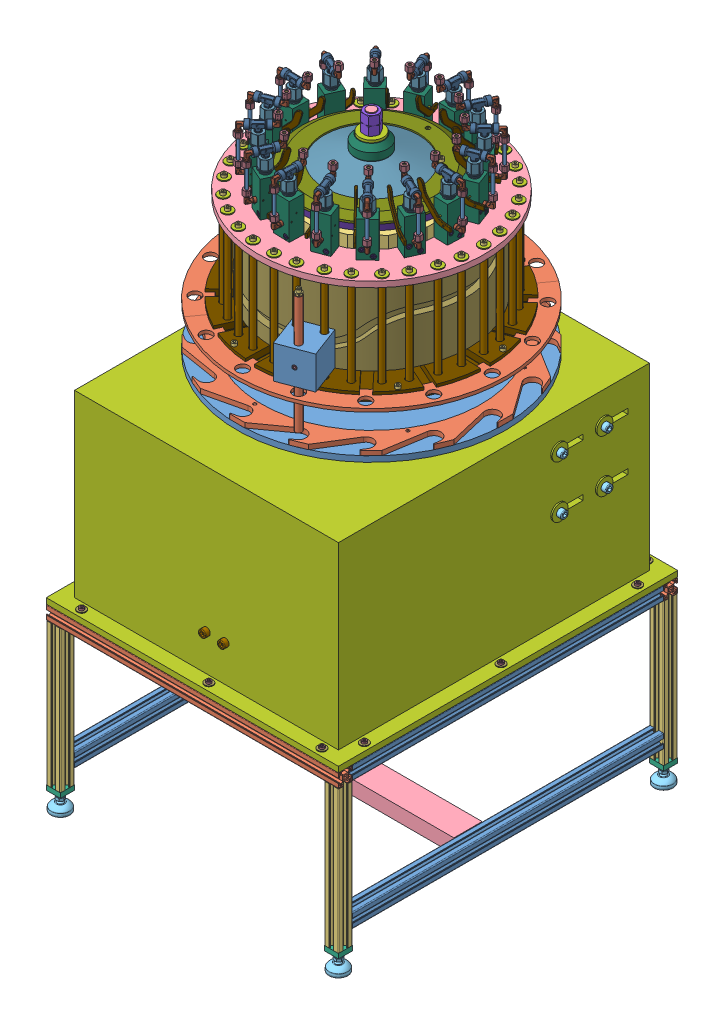
SolidWorks assembly Assieme_FINALE, configuration Default. Lengths in mm.
Overall size (1072.25 1273.72 1072.25).
701 component instances, 78 part files, 66 mates.
Components (placement in the parent):
- SupportoBase_Totale-2: SupportoBase_Totale [Default] at (4.0127 -14.4529 -3.9361) x (0 1 0) z (0 0 1) size (801.2 636.12 736.12)
  - Supporto_base_macchina-1: Supporto_base_macchina [Default] at origin size (378.2 636.12 736.12)
    - profilato_30x30_590-3: profilato_30x30_590 [Default] at (275.414 713.7262 -66.645) size (30 30 660)
    - profilato_30x30_590-5: profilato_30x30_590 [Default] at (275.414 123.7262 -66.645) size (30 30 660)
    - profilato_30x30_550-5: profilato_30x30_550 [Default] at (275.414 703.7262 -716.645) x (1 0 0) z (0 1 0) size (30 30 620)
    - profilato_30x30_550-6: profilato_30x30_550 [Default] at (275.414 703.7262 -26.645) x (1 0 0) z (0 1 0) size (30 30 620)
    - profilato_30x30_272-5: profilato_30x30_272 [Default] at (-16.586 123.7262 -716.645) x (0 0 1) z (-1 0 0) size (30 30 302)
    - profilato_30x30_272-6: profilato_30x30_272 [Default] at (-16.586 713.7262 -716.645) x (0 0 1) z (-1 0 0) size (30 30 302)
    - profilato_30x30_272-7: profilato_30x30_272 [Default] at (235.414 123.7262 -26.645) x (0 0 -1) z (1 0 0) size (30 30 302)
    - profilato_30x30_272-8: profilato_30x30_272 [Default] at (-16.586 713.7262 -26.645) x (0 0 1) z (-1 0 0) size (30 30 302)
    - profilo_U_60x30_490_supporto_base_macchina-1: profilo_U_60x30_490_supporto_base_macchina [Default] at (15.1 707.7262 -323.6583) x (0 0 1) z (0 -1 0) size (60 30 569)
    - profilato_30x30_590-6: profilato_30x30_590 [Default] at (3.414 123.7262 -66.645) size (30 30 660)
    - profilato_30x30_590-7: profilato_30x30_590 [Default] at (3.414 713.7262 -676.645) x (-1 0 0) z (0 0 -1) size (30 30 660)
    - 6322125-1: 6322125 [Default] at (-85.2818 713.7262 -26.645) x (0 0 -1) z (1 0 0) size (40 40 71.2)
    - 6322125-2: 6322125 [Default] at (-85.2818 713.7262 -716.645) x (0 0 -1) z (1 0 0) size (40 40 71.2)
    - 6322125-3: 6322125 [Default] at (-85.2818 123.7262 -26.645) x (0 -0.924225 -0.381849) z (1 0 0) size (40 40 71.2)
    - 6322125-4: 6322125 [Default] at (-85.2818 123.7262 -716.645) x (0 0 -1) z (1 0 0) size (40 40 71.2)
    - tappo_filettato_Supporto_base_macchina-1: tappo_filettato_Supporto_base_macchina [Default] at (-41.586 123.7262 -26.645) x (0 0 1) z (-1 0 0) size (30 30 10.37)
    - tappo_filettato_Supporto_base_macchina-2: tappo_filettato_Supporto_base_macchina [Default] at (-41.586 123.7262 -716.645) x (0 0 1) z (-1 0 0) size (30 30 10.37)
    - tappo_filettato_Supporto_base_macchina-3: tappo_filettato_Supporto_base_macchina [Default] at (-41.586 713.7262 -716.645) x (0 0 1) z (-1 0 0) size (30 30 10.37)
    - tappo_filettato_Supporto_base_macchina-4: tappo_filettato_Supporto_base_macchina [Default] at (-51.586 713.7262 -26.645) x (0 0 -1) z (1 0 0) size (30 30 10.37)
  - assieme_base-1: assieme_base [Default] at (466.8009 1138.7262 -472.0974) x (0 0 -1) z (0 -1 0) size (720 423 620)
    - Supporto di Base per macchina-1: Supporto di Base per macchina [Default] at (-460.4524 -176.3869 1030) size (720 403 620)
    - canotto di supporto-1: canotto di supporto [Default] at (-100.4524 134.8265 740) x (0 1 0) z (-0.866025 0 0.5) size (220 238 238)
    - m10 35mm-7: m10 35mm [ISO 4762 M10 x 35 - 35N] at (4.5476 246.6131 740) x (0 -1 0) z (1 0 0) size (45 16 16)
    - m10 35mm-8: m10 35mm [ISO 4762 M10 x 35 - 35N] at (-47.9524 246.6131 649.0673) x (0 -1 0) z (0.5 0 -0.866025) size (45 16 16)
    - m10 35mm-9: m10 35mm [ISO 4762 M10 x 35 - 35N] at (-152.9524 246.6131 649.0673) x (0 -1 0) z (-0.5 0 -0.866025) size (45 16 16)
    - m10 35mm-10: m10 35mm [ISO 4762 M10 x 35 - 35N] at (-205.4524 246.6131 740) x (0 -1 0) z (-1 0 0) size (45 16 16)
    - m10 35mm-11: m10 35mm [ISO 4762 M10 x 35 - 35N] at (-152.9524 246.6131 830.9327) x (0 -1 0) z (-0.5 0 0.866025) size (45 16 16)
    - m10 35mm-12: m10 35mm [ISO 4762 M10 x 35 - 35N] at (-47.9524 246.6131 830.9327) x (0 -1 0) z (0.5 0 0.866025) size (45 16 16)
    - Traversa di blocco albero-1: Traversa di blocco albero [Default] at (-100.4524 -86.3869 772.5) size (644 42 65)
    - m10 35mm-13: m10 35mm [ISO 4762 M10 x 35 - 35N] at (239.5476 -86.3869 760) x (-1 0 0) z (0 -1 0) size (45 16 16)
    - m10 35mm-16: m10 35mm [ISO 4762 M10 x 35 - 35N] at (239.5476 -86.3869 720) x (-1 0 0) z (0 -1 0) size (45 16 16)
    - m10 35mm-17: m10 35mm [ISO 4762 M10 x 35 - 35N] at (-440.4524 -86.3869 720) x (1 0 0) z (0 1 0) size (45 16 16)
    - m10 35mm-18: m10 35mm [ISO 4762 M10 x 35 - 35N] at (-440.4524 -86.3869 760) x (1 0 0) z (0 1 0) size (45 16 16)
  - DadoT-2: DadoT [Default] at (288.4104 668.7262 -716.645) x (0 0 -1) z (0 -1 0) size (16.5 6 8)
  - DadoT-9: DadoT [Default] at (288.4104 668.7262 -26.645) x (0 0 -1) z (0 -1 0) size (16.5 6 8)
  - DadoT-10: DadoT [Default] at (288.6104 713.7262 -661.645) x (0 1 0) z (0 0 -1) size (16.5 6 8)
  - DadoT-11: DadoT [Default] at (288.6104 713.7262 -371.645) x (0 1 0) z (0 0 -1) size (16.5 6 8)
  - DadoT-12: DadoT [Default] at (288.6104 713.7262 -81.645) x (0 1 0) z (0 0 -1) size (16.5 6 8)
  - DadoT-13: DadoT [Default] at (288.6104 123.7262 -661.645) x (0 1 0) z (0 0 -1) size (16.5 6 8)
  - DadoT-15: DadoT [Default] at (288.6104 123.7262 -371.645) x (0 1 0) z (0 0 -1) size (16.5 6 8)
  - DadoT-17: DadoT [Default] at (288.6104 123.7262 -81.645) x (0 1 0) z (0 0 -1) size (16.5 6 8)
  - RosettaM6-1: RosettaM6 [Washer ISO 7093 - 6] at (302.414 713.7262 -661.645) x (-1 0 0) z (0 0 1) size (1.6 18 18)
  - ViteM6-20-1: ViteM6-20 [ISO 4762 M6 x 20 - 20S] at (308.414 713.7262 -661.645) x (-1 0 0) z (0 0 1) size (26 10 10)
  - RosettaM6-2: RosettaM6 [Washer ISO 7093 - 6] at (302.414 668.7262 -716.645) x (-1 0 0) z (0 0 1) size (1.6 18 18)
  - ViteM6-20-2: ViteM6-20 [ISO 4762 M6 x 20 - 20S] at (308.414 668.7262 -716.645) x (-1 0 0) z (0 0 1) size (26 10 10)
  - RosettaM6-3: RosettaM6 [Washer ISO 7093 - 6] at (302.414 713.7262 -371.645) x (-1 0 0) z (0 0 1) size (1.6 18 18)
  - RosettaM6-4: RosettaM6 [Washer ISO 7093 - 6] at (302.414 713.7262 -81.645) x (-1 0 0) z (0 0 1) size (1.6 18 18)
  - ViteM6-20-3: ViteM6-20 [ISO 4762 M6 x 20 - 20S] at (308.414 713.7262 -371.645) x (-1 0 0) z (0 0 1) size (26 10 10)
  - ViteM6-20-4: ViteM6-20 [ISO 4762 M6 x 20 - 20S] at (308.414 713.7262 -81.645) x (-1 0 0) z (0 0 1) size (26 10 10)
  - RosettaM6-5: RosettaM6 [Washer ISO 7093 - 6] at (302.414 123.7262 -661.645) x (-1 0 0) z (0 0 1) size (1.6 18 18)
  - ViteM6-20-5: ViteM6-20 [ISO 4762 M6 x 20 - 20S] at (308.414 123.7262 -661.645) x (-1 0 0) z (0 0 1) size (26 10 10)
  - RosettaM6-6: RosettaM6 [Washer ISO 7093 - 6] at (302.414 123.7262 -371.645) x (-1 0 0) z (0 0 1) size (1.6 18 18)
  - RosettaM6-7: RosettaM6 [Washer ISO 7093 - 6] at (302.414 123.7262 -81.645) x (-1 0 0) z (0 0 1) size (1.6 18 18)
  - ViteM6-20-6: ViteM6-20 [ISO 4762 M6 x 20 - 20S] at (308.414 123.7262 -371.645) x (-1 0 0) z (0 0 1) size (26 10 10)
  - ViteM6-20-7: ViteM6-20 [ISO 4762 M6 x 20 - 20S] at (308.414 123.7262 -81.645) x (-1 0 0) z (0 0 1) size (26 10 10)
  - ViteM6-20-8: ViteM6-20 [ISO 4762 M6 x 20 - 20S] at (308.414 398.7262 -716.645) x (-1 0 0) z (0 0 1) size (26 10 10)
  - RosettaM6-8: RosettaM6 [Washer ISO 7093 - 6] at (302.414 398.7262 -716.645) x (-1 0 0) z (0 0 1) size (1.6 18 18)
  - DadoT-19: DadoT [Default] at (288.4104 398.7262 -716.645) x (0 0 -1) z (0 -1 0) size (16.5 6 8)
  - DadoT-20: DadoT [Default] at (288.4104 158.7262 -716.645) x (0 0 -1) z (0 -1 0) size (16.5 6 8)
  - RosettaM6-9: RosettaM6 [Washer ISO 7093 - 6] at (302.414 158.7262 -716.645) x (-1 0 0) z (0 0 1) size (1.6 18 18)
  - ViteM6-20-9: ViteM6-20 [ISO 4762 M6 x 20 - 20S] at (308.414 158.7262 -716.645) x (-1 0 0) z (0 0 1) size (26 10 10)
  - DadoT-21: DadoT [Default] at (288.4104 668.7262 -26.645) x (0 0 -1) z (0 -1 0) size (16.5 6 8)
  - RosettaM6-10: RosettaM6 [Washer ISO 7093 - 6] at (302.414 668.7262 -26.645) x (-1 0 0) z (0 0 1) size (1.6 18 18)
  - ViteM6-20-10: ViteM6-20 [ISO 4762 M6 x 20 - 20S] at (308.414 668.7262 -26.645) x (-1 0 0) z (0 0 1) size (26 10 10)
  - DadoT-22: DadoT [Default] at (288.4104 158.7262 -26.645) x (0 0 -1) z (0 -1 0) size (16.5 6 8)
  - RosettaM6-11: RosettaM6 [Washer ISO 7093 - 6] at (302.414 158.7262 -26.645) x (-1 0 0) z (0 0 1) size (1.6 18 18)
  - ViteM6-20-11: ViteM6-20 [ISO 4762 M6 x 20 - 20S] at (308.414 158.7262 -26.645) x (-1 0 0) z (0 0 1) size (26 10 10)
  - ViteM6-20-12: ViteM6-20 [ISO 4762 M6 x 20 - 20S] at (308.414 398.7262 -26.645) x (-1 0 0) z (0 0 1) size (26 10 10)
  - RosettaM6-12: RosettaM6 [Washer ISO 7093 - 6] at (302.414 398.7262 -26.645) x (-1 0 0) z (0 0 1) size (1.6 18 18)
  - DadoT-23: DadoT [Default] at (288.4104 398.7262 -26.645) x (0 0 -1) z (0 -1 0) size (16.5 6 8)
- motoriduttore-1: motoriduttore [Default] at (-164.7135 275.9611 -1137.0941) x (0 0 1) z (-1 0 0) size (200 160 175)
- Assieme_Riduttore-1: Assieme_Riduttore [Default] at (-58.5438 520.923 -522.9431) x (0 1 0) z (-0.993104 0 -0.117237) size (226 168.82 169.04)
  - AlberoRiduttore-1: AlberoRiduttore [Default] at (-61.6906 7.4655 211) size (201 29 29)
  - linguetta_uni6604_b_8x7x50-1: linguetta_uni6604_b_8x7x50 [Default] at (-116.7419 7.4655 226) x (1 0 0) z (0 1 0) size (50 7 8)
  - linguetta_uni6604_b_8x7x35-1: linguetta_uni6604_b_8x7x35 [Default] at (-33.7419 7.4655 226.5) x (1 0 0) z (0 1 0) size (35 7 8)
  - linguetta_uni6604_b_8x7x35-2: linguetta_uni6604_b_8x7x35 [Default] at (41.2581 7.4655 226.5) x (1 0 0) z (0 1 0) size (35 7 8)
  - ASSIEME-LASS-90-VERS-B-O-25-3D.step-1: ASSIEME-LASS-90-VERS-B-O-25-3D.step [Default] at (-111.3519 -70.5563 279.3493) x (-1 0 0) z (0 0.707107 -0.707107) size (64.28 105 105)
  - Rondella di fermo-1: Rondella di fermo [Default] at (-122.7419 7.4655 211) x (0 0.707107 -0.707107) z (-1 0 0) size (36 36 3)
  - M8 25 mm-1: M8 25 mm [ISO 4762 M8 x 25 - 25N] at (92.2581 7.4655 211) x (-1 0 0) z (0 1 0) size (33 13 13)
  - M8 25 mm-2: M8 25 mm [ISO 4762 M8 x 25 - 25N] at (-133.7419 7.4655 211) x (1 0 0) z (0 -0.707107 0.707107) size (33 13 13)
  - M6 16mm-3: M6 16mm [ISO 4762 M6 x 16 - 16N] at (-44.8119 40.5589 196.8286) x (-1 0 0) z (0 0.935687 0.352831) size (22 10 10)
  - M6 16mm-14: M6 16mm [ISO 4762 M6 x 16 - 16N] at (-44.8119 11.7394 175.2546) x (-1 0 0) z (0 0.773404 -0.633913) size (22 10 10)
  - M6 16mm-15: M6 16mm [ISO 4762 M6 x 16 - 16N] at (-44.8119 -21.354 189.426) x (-1 0 0) z (0 -0.162283 -0.986744) size (22 10 10)
  - M6 16mm-16: M6 16mm [ISO 4762 M6 x 16 - 16N] at (-44.8119 -25.6279 225.1714) x (-1 0 0) z (0 -0.935687 -0.352831) size (22 10 10)
  - M6 16mm-17: M6 16mm [ISO 4762 M6 x 16 - 16N] at (-44.8119 3.1916 246.7454) x (-1 0 0) z (0 -0.773404 0.633913) size (22 10 10)
  - M6 16mm-18: M6 16mm [ISO 4762 M6 x 16 - 16N] at (-44.8119 36.285 232.574) x (-1 0 0) z (0 0.162283 0.986744) size (22 10 10)
  - Parte1^Assieme_Riduttore-1: Parte1^Assieme_Riduttore [Default] at origin (virtual)
  - ruota dentata m22-4: ruota dentata m22 [Chain wheel ISO - 22Z 10A-1 --22SA36.0N] at (-59.7419 7.4655 211) x (1 0 0) z (0 -0.599278 0.800541) size (8.93 120.13 121.23)
  - Rondella di fermo-2: Rondella di fermo [Default] at (84.2581 7.4655 211) x (0 0 1) z (-1 0 0) size (36 36 3)
- M10 50mm-1: M10 50mm [ISO 4762 M10 x 50 - 50N] at (-121.7135 603.4611 -513.0941) x (-1 0 0) z (0 -0.924225 -0.381849) size (60 16 16)
- M10 50mm-2: M10 50mm [ISO 4762 M10 x 50 - 50N] at (-121.7135 492.4611 -513.0941) x (-1 0 0) z (0 0 1) size (60 16 16)
- M10 50mm-5: M10 50mm [ISO 4762 M10 x 50 - 50N] at (-121.7135 603.4611 -608.0941) x (-1 0 0) z (0 0 1) size (60 16 16)
- M10 50mm-4: M10 50mm [ISO 4762 M10 x 50 - 50N] at (-121.7135 492.4611 -608.0941) x (-1 0 0) z (0 0 1) size (60 16 16)
- DADO M10-9: DADO M10 [ISO - 4033 - M10 - W - N] at (-174.0135 603.4611 -608.0941) x (0 0 1) z (-1 0 0) size (16 18.48 9.3)
- DADO M10-8: DADO M10 [ISO - 4033 - M10 - W - N] at (-174.0135 603.4611 -513.0941) x (0 0 1) z (-1 0 0) size (16 18.48 9.3)
- DADO M10-7: DADO M10 [ISO - 4033 - M10 - W - N] at (-174.0135 492.4611 -608.0941) x (0 0 1) z (-1 0 0) size (16 18.48 9.3)
- DADO M10-10: DADO M10 [ISO - 4033 - M10 - W - N] at (-174.0135 492.4611 -513.0941) x (0 0 1) z (-1 0 0) size (16 18.48 9.3)
- rondella M10-9: rondella M10 [Washer ISO 7094 - 10] at (-134.7135 603.4611 -513.0941) x (-1 0 0) z (0 0.924225 0.381849) size (3 34 34)
- rondella M10-10: rondella M10 [Washer ISO 7094 - 10] at (-134.7135 492.4611 -513.0941) x (-1 0 0) z (0 0 1) size (3 34 34)
- rondella M10-12: rondella M10 [Washer ISO 7094 - 10] at (-134.7135 492.4611 -608.0941) x (-1 0 0) z (0 0 1) size (3 34 34)
- rondella M10-11: rondella M10 [Washer ISO 7094 - 10] at (-134.7135 603.4611 -608.0941) x (-1 0 0) z (0 0 1) size (3 34 34)
- catena_maschio-1: catena_maschio [Default] at (-321.9473 463.4961 -580.6395) x (-0.810007 0 0.58642) z (0 1 0) size (28.67 12.73 20.3)
- catena_femmina-1: catena_femmina [Default] at (-334.299 463.4961 -567.4631) x (0.810007 0 -0.58642) z (0 1 0) size (30.04 14.2 13.87)
  - ansi_50_02-1: ansi_50_02 [Default] at (17.7318 3.4296 0) x (1 0 0) z (0 0 -1) size (30.04 14.2 13.87)
  - ansi_50_03-1: ansi_50_03 [Default] at (17.7318 3.4296 -0.11) x (1 0 0) z (0 0 -1) size (10.16 10.16 9.46)
  - ansi_50_04-1: ansi_50_04 [Default] at (17.7318 3.4296 0.11) x (1 0 0) z (0 0 -1) size (10.16 10.16 9.46)
- rondella M8-1: rondella M8 [ISO 10673-9.3-S] at (-394.7135 376.9611 -360.5811) x (0 -1 0) z (-1 0 0) size (2 18 18)
- rondella M8-2: rondella M8 [ISO 10673-9.3-S] at (-394.7135 376.9611 -390.5811) x (0 -1 0) z (-1 0 0) size (2 18 18)
- M8 25 mm-1: M8 25 mm [ISO 4762 M8 x 25 - 25N] at (-394.7135 368.9611 -390.5811) x (0 1 0) z (0.5 0 0.866025) size (33 13 13)
- M8 25 mm-2: M8 25 mm [ISO 4762 M8 x 25 - 25N] at (-394.7135 366.9611 -360.5811) x (0 1 0) z (-0.5 0 -0.866025) size (33 13 13)
- assieme parte rotante-2: assieme parte rotante [Default] at (-160.1634 623.9178 -718.4345) x (0 1 0) z (-0.527591 0 0.849499) size (749.63 778.63 778.63)
  - albero rotazione piatti-1: albero rotazione piatti [Default] at (60.413 18.3637 415) size (415 200 200)
  - seger 100mm-2: seger 100mm [KS 1336 E - 100] at (-146.4567 18.3637 415) x (0 0 -1) z (1 0 0) size (107.55 112.98 3)
  - SKF - 6020 - 20,DE,NC,20_68-1: SKF - 6020 - 20,DE,NC,20_68 [SKF - 6020 - 20,DE,NC,20_68] at (-131.4567 18.3637 415) x (1 0 0) z (0 -0.434476 -0.900684) size (24 150 150)
  - calettatore d95-1: calettatore d95 [Default] at (-173.8867 18.3637 415) size (39.5 135 135)
  - Chain wheel ISO - 50Z 10A-1-1: Chain wheel ISO - 50Z 10A-1 [Chain wheel ISO - 50Z 10A-1 --50SB120H25L95.0N] at (-164.8867 18.3637 415) size (28.93 262.06 262.51)
  - Disco supporto montaggio e Colonne-1: Disco supporto montaggio e Colonne [Default] at (204.0433 18.3637 415) x (0 -0.866025 -0.5) z (1 0 0) size (499.6 499.6 29)
  - SKF - 6020 - 20,DE,NC,20_68-2: SKF - 6020 - 20,DE,NC,20_68 [SKF - 6020 - 20,DE,NC,20_68] at (62.0433 18.3637 415) x (1 0 0) z (0 -0.432628 -0.901573) size (24 150 150)
  - piatto rotante porta tappi-1: piatto rotante porta tappi [Default] at (99.0433 18.3637 415) x (0 0 -1) z (1 0 0) size (570 570 20.57)
  - disco trasportatore tappi 31-1: disco trasportatore tappi 31 [Default] at (111.0433 18.3637 415) x (0 0.5 -0.866025) z (1 0 0) size (570 570 10.42)
  - Distributore Rotante-1: Distributore Rotante [Default] at (425.0433 18.3637 415) x (0 0.130526 -0.991445) z (1 0 0) size (310 310 25.54)
  - disco trascinato porta distributore vuoto-1: disco trascinato porta distributore vuoto [Default] at (400.0433 18.3637 415) x (0 -0.130526 0.991445) z (-1 0 0) size (480 480 50)
  - m12 35mm-1: m12 35mm [ISO 4762 M12 x 35 - 35N] at (376.0433 -45.1046 366.2991) x (1 0 0) z (0 -0.5 0.866025) size (47 18 18)
  - m12 90mm-3: m12 90mm [ISO 4762 M12 x 90 - 90N] at (203.0433 -21.6363 345.718) x (-1 0 0) z (0 -0.5 0.866025) size (102 18 18)
  - rondella M6-90: rondella M6 [Washer ISO 7094 - 6] at (99.0433 -101.6363 207.1539) x (1 0 0) z (0 -1 0) size (2 22 22)
  - M6 20mm-1: M6 20mm [ISO 4762 M6 x 20 - 20N] at (91.0433 -101.6363 207.1539) x (1 0 0) z (0 0.5 0.866025) size (26 10 10)
  - m12 35mm-2: m12 35mm [ISO 4762 M12 x 35 - 35N] at (376.0433 28.8058 335.6844) x (1 0 0) z (0 -1 0) size (47 18 18)
  - m12 35mm-3: m12 35mm [ISO 4762 M12 x 35 - 35N] at (376.0433 92.2741 384.3853) x (1 0 0) z (0 -0.5 -0.866025) size (47 18 18)
  - m12 35mm-4: m12 35mm [ISO 4762 M12 x 35 - 35N] at (376.0433 81.832 463.7009) x (1 0 0) z (0 0.5 -0.866025) size (47 18 18)
  - m12 35mm-5: m12 35mm [ISO 4762 M12 x 35 - 35N] at (376.0433 7.9216 494.3156) x (1 0 0) z (0 1 0) size (47 18 18)
  - m12 35mm-6: m12 35mm [ISO 4762 M12 x 35 - 35N] at (376.0433 -55.5467 445.6147) x (1 0 0) z (0 0.5 0.866025) size (47 18 18)
  - rondella M6-91: rondella M6 [Washer ISO 7094 - 6] at (99.0433 138.3637 207.1539) x (1 0 0) z (0 -0.5 -0.866025) size (2 22 22)
  - rondella M6-92: rondella M6 [Washer ISO 7094 - 6] at (99.0433 258.3637 415) x (1 0 0) z (0 0.5 -0.866025) size (2 22 22)
  - rondella M6-93: rondella M6 [Washer ISO 7094 - 6] at (99.0433 138.3637 622.8461) x (1 0 0) z (0 1 0) size (2 22 22)
  - rondella M6-94: rondella M6 [Washer ISO 7094 - 6] at (99.0433 -101.6363 622.8461) x (1 0 0) z (0 0.5 0.866025) size (2 22 22)
  - rondella M6-95: rondella M6 [Washer ISO 7094 - 6] at (99.0433 -221.6363 415) x (1 0 0) z (0 -0.5 0.866025) size (2 22 22)
  - M6 20mm-2: M6 20mm [ISO 4762 M6 x 20 - 20N] at (91.0433 138.3637 207.1539) x (1 0 0) z (0 -0.5 0.866025) size (26 10 10)
  - M6 20mm-3: M6 20mm [ISO 4762 M6 x 20 - 20N] at (91.0433 258.3637 415) x (1 0 0) z (0 -1 0) size (26 10 10)
  - M6 20mm-4: M6 20mm [ISO 4762 M6 x 20 - 20N] at (91.0433 138.3637 622.8461) x (1 0 0) z (0 -0.5 -0.866025) size (26 10 10)
  - M6 20mm-5: M6 20mm [ISO 4762 M6 x 20 - 20N] at (91.0433 -101.6363 622.8461) x (1 0 0) z (0 0.5 -0.866025) size (26 10 10)
  - M6 20mm-6: M6 20mm [ISO 4762 M6 x 20 - 20N] at (91.0433 -221.6363 415) x (1 0 0) z (0 1 0) size (26 10 10)
  - m12 90mm-4: m12 90mm [ISO 4762 M12 x 90 - 90N] at (203.0433 58.3637 345.718) x (-1 0 0) z (0 -1 0) size (102 18 18)
  - m12 90mm-5: m12 90mm [ISO 4762 M12 x 90 - 90N] at (203.0433 98.3637 415) x (-1 0 0) z (0 -0.5 -0.866025) size (102 18 18)
  - m12 90mm-6: m12 90mm [ISO 4762 M12 x 90 - 90N] at (203.0433 58.3637 484.282) x (-1 0 0) z (0 0.5 -0.866025) size (102 18 18)
  - m12 90mm-7: m12 90mm [ISO 4762 M12 x 90 - 90N] at (203.0433 -21.6363 484.282) x (-1 0 0) z (0 1 0) size (102 18 18)
  - m12 90mm-8: m12 90mm [ISO 4762 M12 x 90 - 90N] at (203.0433 -61.6363 415) x (-1 0 0) z (0 0.5 0.866025) size (102 18 18)
  - asta scorrimento carello-1: asta scorrimento carello [Default] at (287.5433 70.1437 197.9013) x (0 0 -1) z (1 0 0) size (12 12 225)
  - rondella M6-74: rondella M6 [Washer ISO 7094 - 6] at (175.0433 70.1437 197.9013) x (1 0 0) z (0 -1 0) size (2 22 22)
  - M6 16mm-1: M6 16mm [ISO 4762 M6 x 16 - 16N] at (167.0433 70.1437 197.9013) size (22 10 10)
  - M6 16mm-2: M6 16mm [ISO 4762 M6 x 16 - 16N] at (408.0433 70.1437 197.9013) x (-1 0 0) z (0 0 -1) size (22 10 10)
  - rondella M6-96: rondella M6 [Washer ISO 7094 - 6] at (400.0433 70.1437 197.9013) x (-1 0 0) z (0 1 0) size (2 22 22)
  - rondella M6-112: rondella M6 [Washer ISO 7094 - 6] at (175.0433 24.5373 191.8971) x (1 0 0) z (0 -0.965926 -0.258819) size (2 22 22)
  - M6 16mm-3: M6 16mm [ISO 4762 M6 x 16 - 16N] at (167.0433 24.5373 191.8971) x (1 0 0) z (0 0.258819 -0.965926) size (22 10 10)
  - asta scorrimento carello-2: asta scorrimento carello [Default] at (287.5433 24.5373 191.8971) x (0 0.258819 -0.965926) z (-1 0 0) size (12 12 225)
  - rondella M6-128: rondella M6 [Washer ISO 7094 - 6] at (400.0433 24.5373 191.8971) x (-1 0 0) z (0 0.965926 0.258819) size (2 22 22)
  - M6 16mm-4: M6 16mm [ISO 4762 M6 x 16 - 16N] at (408.0433 24.5373 191.8971) x (-1 0 0) z (0 -0.258819 0.965926) size (22 10 10)
  - AssiemeValvola-1: AssiemeValvola [Default] at (515.3257 103.3637 267.7757) x (0 -0.5 0.866025) z (0 0.866025 0.5) size (90.26 138.63 38)
    - RaccordoT-1: RaccordoT [Default] at origin size (43 29.75 16.5)
    - Raccordo a L-1: Raccordo a L [Default] at (-30 0 0) x (0 -1 0) z (0 0 -1) size (28.34 25.51 14.01)
      - 1809_06_10_01-1: 1809_06_10_01 [Default] at origin size (22.49 23 10)
      - 1809_06_10_02-1: 1809_06_10_02 [Default] at origin size (6.5 8.5 8.5)
      - 1809_06_10_03-1: 1809_06_10_03 [Default] at origin size (11.02 15.01 14.01)
    - Raccordo a L-2: Raccordo a L [Default] at (30 0 0) x (0 1 0) z (0 0 -1) size (28.34 25.51 14.01)
      - 1809_06_10_01-1: 1809_06_10_01 [Default] at origin size (22.49 23 10)
      - 1809_06_10_02-1: 1809_06_10_02 [Default] at origin size (6.5 8.5 8.5)
      - 1809_06_10_03-1: 1809_06_10_03 [Default] at origin size (11.02 15.01 14.01)
    - TappoChiusura-1: TappoChiusura [Default] at (0 -32 0) x (0 -1 0) z (0 0 1) size (38.28 26.74 26.74)
    - CorpoValvola-1: CorpoValvola [Default] at (-15 -115.2824 0) size (30 75 34)
    - Raccordo a L-3: Raccordo a L [Default] at (-30 -88.2824 0) x (0 1 0) z (0 0 1) size (28.34 25.51 14.01)
      - 1809_06_10_01-1: 1809_06_10_01 [Default] at origin size (22.49 23 10)
      - 1809_06_10_02-1: 1809_06_10_02 [Default] at origin size (6.5 8.5 8.5)
      - 1809_06_10_03-1: 1809_06_10_03 [Default] at origin size (11.02 15.01 14.01)
    - Spina_3x38-1: Spina_3x38 [Default] at (0 -68.2824 -21) x (-1 0 0) z (0 0 1) size (3 3 38)
    - Spina_3x38-2: Spina_3x38 [Default] at (-10 -80.2824 -21) x (0.996193 0.087174 0) z (0 0 1) size (3 3 38)
    - M5 40mm-3: M5 40mm [ISO 4762 M5 x 40 - 40N] at (-14.6 -108.7824 9) size (45 8.5 8.5)
    - M5 40mm-2: M5 40mm [ISO 4762 M5 x 40 - 40N] at (-14.6 -96.7824 -9) size (45 8.5 8.5)
    - LevaValvola-1: LevaValvola [Default] at (-24.507 -86.571 -17) x (0.996193 0.087174 0) z (0 0 1) size (77.55 60.2 4)
    - Tubo-1: Tubo [Default] at (-30 -15.9665 0) x (1 0 0) z (0 -1 0) size (6 6 56.4)
  - M6 16mm-5: M6 16mm [ISO 4762 M6 x 16 - 16N] at (167.0433 -16.8778 194.6116) x (1 0 0) z (0 0.382683 0.92388) size (22 10 10)
  - M6 16mm-6: M6 16mm [ISO 4762 M6 x 16 - 16N] at (167.0433 -98.5342 224.874) x (1 0 0) z (0 0.707107 0.707107) size (22 10 10)
  - M6 16mm-7: M6 16mm [ISO 4762 M6 x 16 - 16N] at (167.0433 -162.3939 284.0814) x (1 0 0) z (0 0.92388 0.382683) size (22 10 10)
  - M6 16mm-8: M6 16mm [ISO 4762 M6 x 16 - 16N] at (167.0433 -198.735 363.22) x (1 0 0) z (0 1 0) size (22 10 10)
  - M6 16mm-9: M6 16mm [ISO 4762 M6 x 16 - 16N] at (167.0433 -202.0247 450.2415) x (1 0 0) z (0 0.92388 -0.382683) size (22 10 10)
  - M6 16mm-10: M6 16mm [ISO 4762 M6 x 16 - 16N] at (167.0433 -171.7623 531.8979) x (1 0 0) z (0 0.707107 -0.707107) size (22 10 10)
  - M6 16mm-11: M6 16mm [ISO 4762 M6 x 16 - 16N] at (167.0433 -112.5549 595.7576) x (1 0 0) z (0 0.382683 -0.92388) size (22 10 10)
  - M6 16mm-12: M6 16mm [ISO 4762 M6 x 16 - 16N] at (167.0433 -33.4163 632.0987) x (1 0 0) z (0 0 -1) size (22 10 10)
  - M6 16mm-13: M6 16mm [ISO 4762 M6 x 16 - 16N] at (167.0433 53.6052 635.3884) x (1 0 0) z (0 -0.382683 -0.92388) size (22 10 10)
  - M6 16mm-14: M6 16mm [ISO 4762 M6 x 16 - 16N] at (167.0433 135.2616 605.126) x (1 0 0) z (0 -0.707107 -0.707107) size (22 10 10)
  - M6 16mm-15: M6 16mm [ISO 4762 M6 x 16 - 16N] at (167.0433 199.1213 545.9186) x (1 0 0) z (0 -0.92388 -0.382683) size (22 10 10)
  - M6 16mm-16: M6 16mm [ISO 4762 M6 x 16 - 16N] at (167.0433 235.4624 466.78) x (1 0 0) z (0 -1 0) size (22 10 10)
  - M6 16mm-17: M6 16mm [ISO 4762 M6 x 16 - 16N] at (167.0433 238.7521 379.7585) x (1 0 0) z (0 -0.92388 0.382683) size (22 10 10)
  - M6 16mm-18: M6 16mm [ISO 4762 M6 x 16 - 16N] at (167.0433 208.4897 298.1021) x (1 0 0) z (0 -0.707107 0.707107) size (22 10 10)
  - M6 16mm-19: M6 16mm [ISO 4762 M6 x 16 - 16N] at (167.0433 149.2823 234.2424) x (1 0 0) z (0 -0.382683 0.92388) size (22 10 10)
  - rondella M6-75: rondella M6 [Washer ISO 7094 - 6] at (175.0433 -16.8778 194.6116) x (1 0 0) z (0 -0.92388 0.382683) size (2 22 22)
  - rondella M6-76: rondella M6 [Washer ISO 7094 - 6] at (175.0433 -98.5342 224.874) x (1 0 0) z (0 -0.707107 0.707107) size (2 22 22)
  - rondella M6-77: rondella M6 [Washer ISO 7094 - 6] at (175.0433 -162.3939 284.0814) x (1 0 0) z (0 -0.382683 0.92388) size (2 22 22)
  - rondella M6-78: rondella M6 [Washer ISO 7094 - 6] at (175.0433 -198.735 363.22) size (2 22 22)
  - rondella M6-79: rondella M6 [Washer ISO 7094 - 6] at (175.0433 -202.0247 450.2415) x (1 0 0) z (0 0.382683 0.92388) size (2 22 22)
  - rondella M6-80: rondella M6 [Washer ISO 7094 - 6] at (175.0433 -171.7623 531.8979) x (1 0 0) z (0 0.707107 0.707107) size (2 22 22)
  - rondella M6-81: rondella M6 [Washer ISO 7094 - 6] at (175.0433 -112.5549 595.7576) x (1 0 0) z (0 0.92388 0.382683) size (2 22 22)
  - rondella M6-82: rondella M6 [Washer ISO 7094 - 6] at (175.0433 -33.4163 632.0987) x (1 0 0) z (0 1 0) size (2 22 22)
  - rondella M6-83: rondella M6 [Washer ISO 7094 - 6] at (175.0433 53.6052 635.3884) x (1 0 0) z (0 0.92388 -0.382683) size (2 22 22)
  - rondella M6-84: rondella M6 [Washer ISO 7094 - 6] at (175.0433 135.2616 605.126) x (1 0 0) z (0 0.707107 -0.707107) size (2 22 22)
  - rondella M6-85: rondella M6 [Washer ISO 7094 - 6] at (175.0433 199.1213 545.9186) x (1 0 0) z (0 0.382683 -0.92388) size (2 22 22)
  - rondella M6-86: rondella M6 [Washer ISO 7094 - 6] at (175.0433 235.4624 466.78) x (1 0 0) z (0 0 -1) size (2 22 22)
  - rondella M6-87: rondella M6 [Washer ISO 7094 - 6] at (175.0433 238.7521 379.7585) x (1 0 0) z (0 -0.382683 -0.92388) size (2 22 22)
  - rondella M6-88: rondella M6 [Washer ISO 7094 - 6] at (175.0433 208.4897 298.1021) x (1 0 0) z (0 -0.707107 -0.707107) size (2 22 22)
  - rondella M6-89: rondella M6 [Washer ISO 7094 - 6] at (175.0433 149.2823 234.2424) x (1 0 0) z (0 -0.92388 -0.382683) size (2 22 22)
  - asta scorrimento carello-3: asta scorrimento carello [Default] at (287.5433 -16.8778 194.6116) x (0 -0.382683 -0.92388) z (1 0 0) size (12 12 225)
  - asta scorrimento carello-4: asta scorrimento carello [Default] at (287.5433 -98.5342 224.874) x (0 -0.707107 -0.707107) z (1 0 0) size (12 12 225)
  - asta scorrimento carello-5: asta scorrimento carello [Default] at (287.5433 -162.3939 284.0814) x (0 -0.92388 -0.382683) z (1 0 0) size (12 12 225)
  - asta scorrimento carello-6: asta scorrimento carello [Default] at (287.5433 -198.735 363.22) x (0 -1 0) z (1 0 0) size (12 12 225)
  - asta scorrimento carello-7: asta scorrimento carello [Default] at (287.5433 -202.0247 450.2415) x (0 -0.92388 0.382683) z (1 0 0) size (12 12 225)
  - asta scorrimento carello-8: asta scorrimento carello [Default] at (287.5433 -171.7623 531.8979) x (0 -0.707107 0.707107) z (1 0 0) size (12 12 225)
  - asta scorrimento carello-9: asta scorrimento carello [Default] at (287.5433 -112.5549 595.7576) x (0 -0.382683 0.92388) z (1 0 0) size (12 12 225)
  - asta scorrimento carello-10: asta scorrimento carello [Default] at (287.5433 -33.4163 632.0987) x (0 0 1) z (1 0 0) size (12 12 225)
  - asta scorrimento carello-11: asta scorrimento carello [Default] at (287.5433 53.6052 635.3884) x (0 0.382683 0.92388) z (1 0 0) size (12 12 225)
  - asta scorrimento carello-12: asta scorrimento carello [Default] at (287.5433 135.2616 605.126) x (0 0.707107 0.707107) z (1 0 0) size (12 12 225)
  - asta scorrimento carello-13: asta scorrimento carello [Default] at (287.5433 199.1213 545.9186) x (0 0.92388 0.382683) z (1 0 0) size (12 12 225)
  - asta scorrimento carello-14: asta scorrimento carello [Default] at (287.5433 235.4624 466.78) x (0 1 0) z (1 0 0) size (12 12 225)
  - asta scorrimento carello-15: asta scorrimento carello [Default] at (287.5433 238.7521 379.7585) x (0 0.92388 -0.382683) z (1 0 0) size (12 12 225)
  - asta scorrimento carello-16: asta scorrimento carello [Default] at (287.5433 208.4897 298.1021) x (0 0.707107 -0.707107) z (1 0 0) size (12 12 225)
  - asta scorrimento carello-17: asta scorrimento carello [Default] at (287.5433 149.2823 234.2424) x (0 0.382683 -0.92388) z (1 0 0) size (12 12 225)
  - M6 16mm-20: M6 16mm [ISO 4762 M6 x 16 - 16N] at (408.0433 -16.8778 194.6116) x (-1 0 0) z (0 -0.382683 -0.92388) size (22 10 10)
  - M6 16mm-21: M6 16mm [ISO 4762 M6 x 16 - 16N] at (408.0433 -98.5342 224.874) x (-1 0 0) z (0 -0.707107 -0.707107) size (22 10 10)
  - M6 16mm-22: M6 16mm [ISO 4762 M6 x 16 - 16N] at (408.0433 -162.3939 284.0814) x (-1 0 0) z (0 -0.92388 -0.382683) size (22 10 10)
  - M6 16mm-23: M6 16mm [ISO 4762 M6 x 16 - 16N] at (408.0433 -198.735 363.22) x (-1 0 0) z (0 -1 0) size (22 10 10)
  - M6 16mm-24: M6 16mm [ISO 4762 M6 x 16 - 16N] at (408.0433 -202.0247 450.2415) x (-1 0 0) z (0 -0.92388 0.382683) size (22 10 10)
  - M6 16mm-25: M6 16mm [ISO 4762 M6 x 16 - 16N] at (408.0433 -171.7623 531.8979) x (-1 0 0) z (0 -0.707107 0.707107) size (22 10 10)
  - M6 16mm-26: M6 16mm [ISO 4762 M6 x 16 - 16N] at (408.0433 -112.5549 595.7576) x (-1 0 0) z (0 -0.382683 0.92388) size (22 10 10)
  - M6 16mm-27: M6 16mm [ISO 4762 M6 x 16 - 16N] at (408.0433 -33.4163 632.0987) x (-1 0 0) z (0 0 1) size (22 10 10)
  - M6 16mm-28: M6 16mm [ISO 4762 M6 x 16 - 16N] at (408.0433 53.6052 635.3884) x (-1 0 0) z (0 0.382683 0.92388) size (22 10 10)
  - M6 16mm-29: M6 16mm [ISO 4762 M6 x 16 - 16N] at (408.0433 135.2616 605.126) x (-1 0 0) z (0 0.707107 0.707107) size (22 10 10)
  - M6 16mm-30: M6 16mm [ISO 4762 M6 x 16 - 16N] at (408.0433 199.1213 545.9186) x (-1 0 0) z (0 0.92388 0.382683) size (22 10 10)
  - M6 16mm-31: M6 16mm [ISO 4762 M6 x 16 - 16N] at (408.0433 235.4624 466.78) x (-1 0 0) z (0 1 0) size (22 10 10)
  - M6 16mm-32: M6 16mm [ISO 4762 M6 x 16 - 16N] at (408.0433 238.7521 379.7585) x (-1 0 0) z (0 0.92388 -0.382683) size (22 10 10)
  - M6 16mm-33: M6 16mm [ISO 4762 M6 x 16 - 16N] at (408.0433 208.4897 298.1021) x (-1 0 0) z (0 0.707107 -0.707107) size (22 10 10)
  - M6 16mm-34: M6 16mm [ISO 4762 M6 x 16 - 16N] at (408.0433 149.2823 234.2424) x (-1 0 0) z (0 0.382683 -0.92388) size (22 10 10)
  - rondella M6-97: rondella M6 [Washer ISO 7094 - 6] at (400.0433 -16.8778 194.6116) x (-1 0 0) z (0 0.92388 -0.382683) size (2 22 22)
  - rondella M6-98: rondella M6 [Washer ISO 7094 - 6] at (400.0433 -98.5342 224.874) x (-1 0 0) z (0 0.707107 -0.707107) size (2 22 22)
  - rondella M6-99: rondella M6 [Washer ISO 7094 - 6] at (400.0433 -162.3939 284.0814) x (-1 0 0) z (0 0.382683 -0.92388) size (2 22 22)
  - rondella M6-100: rondella M6 [Washer ISO 7094 - 6] at (400.0433 -198.735 363.22) x (-1 0 0) z (0 0 -1) size (2 22 22)
  - rondella M6-101: rondella M6 [Washer ISO 7094 - 6] at (400.0433 -202.0247 450.2415) x (-1 0 0) z (0 -0.382683 -0.92388) size (2 22 22)
  - rondella M6-102: rondella M6 [Washer ISO 7094 - 6] at (400.0433 -171.7623 531.8979) x (-1 0 0) z (0 -0.707107 -0.707107) size (2 22 22)
  - rondella M6-103: rondella M6 [Washer ISO 7094 - 6] at (400.0433 -112.5549 595.7576) x (-1 0 0) z (0 -0.92388 -0.382683) size (2 22 22)
  - rondella M6-104: rondella M6 [Washer ISO 7094 - 6] at (400.0433 -33.4163 632.0987) x (-1 0 0) z (0 -1 0) size (2 22 22)
  - rondella M6-105: rondella M6 [Washer ISO 7094 - 6] at (400.0433 53.6052 635.3884) x (-1 0 0) z (0 -0.92388 0.382683) size (2 22 22)
  - rondella M6-106: rondella M6 [Washer ISO 7094 - 6] at (400.0433 135.2616 605.126) x (-1 0 0) z (0 -0.707107 0.707107) size (2 22 22)
  - rondella M6-107: rondella M6 [Washer ISO 7094 - 6] at (400.0433 199.1213 545.9186) x (-1 0 0) z (0 -0.382683 0.92388) size (2 22 22)
  - rondella M6-108: rondella M6 [Washer ISO 7094 - 6] at (400.0433 235.4624 466.78) x (-1 0 0) z (0 0 1) size (2 22 22)
  - rondella M6-109: rondella M6 [Washer ISO 7094 - 6] at (400.0433 238.7521 379.7585) x (-1 0 0) z (0 0.382683 0.92388) size (2 22 22)
  - rondella M6-110: rondella M6 [Washer ISO 7094 - 6] at (400.0433 208.4897 298.1021) x (-1 0 0) z (0 0.707107 0.707107) size (2 22 22)
  - rondella M6-111: rondella M6 [Washer ISO 7094 - 6] at (400.0433 149.2823 234.2424) x (-1 0 0) z (0 0.92388 0.382683) size (2 22 22)
  - rondella M6-113: rondella M6 [Washer ISO 7094 - 6] at (175.0433 -61.3104 206.5173) x (1 0 0) z (0 -0.991445 0.130526) size (2 22 22)
  - rondella M6-114: rondella M6 [Washer ISO 7094 - 6] at (175.0433 -135.0285 252.8771) x (1 0 0) z (0 -0.866025 0.5) size (2 22 22)
  - rondella M6-115: rondella M6 [Washer ISO 7094 - 6] at (175.0433 -185.3939 323.9186) x (1 0 0) z (0 -0.608761 0.793353) size (2 22 22)
  - rondella M6-116: rondella M6 [Washer ISO 7094 - 6] at (175.0433 -204.7392 408.8264) x (1 0 0) z (0 -0.258819 0.965926) size (2 22 22)
  - rondella M6-117: rondella M6 [Washer ISO 7094 - 6] at (175.0433 -190.119 494.6741) x (1 0 0) z (0 0.130526 0.991445) size (2 22 22)
  - rondella M6-118: rondella M6 [Washer ISO 7094 - 6] at (175.0433 -143.7592 568.3922) x (1 0 0) z (0 0.5 0.866025) size (2 22 22)
  - rondella M6-119: rondella M6 [Washer ISO 7094 - 6] at (175.0433 -72.7177 618.7576) x (1 0 0) z (0 0.793353 0.608761) size (2 22 22)
  - rondella M6-120: rondella M6 [Washer ISO 7094 - 6] at (175.0433 12.1901 638.1029) x (1 0 0) z (0 0.965926 0.258819) size (2 22 22)
  - rondella M6-121: rondella M6 [Washer ISO 7094 - 6] at (175.0433 98.0378 623.4827) x (1 0 0) z (0 0.991445 -0.130526) size (2 22 22)
  - rondella M6-122: rondella M6 [Washer ISO 7094 - 6] at (175.0433 171.7559 577.1229) x (1 0 0) z (0 0.866025 -0.5) size (2 22 22)
  - rondella M6-123: rondella M6 [Washer ISO 7094 - 6] at (175.0433 222.1213 506.0814) x (1 0 0) z (0 0.608761 -0.793353) size (2 22 22)
  - rondella M6-124: rondella M6 [Washer ISO 7094 - 6] at (175.0433 241.4666 421.1736) x (1 0 0) z (0 0.258819 -0.965926) size (2 22 22)
  - rondella M6-125: rondella M6 [Washer ISO 7094 - 6] at (175.0433 226.8464 335.3259) x (1 0 0) z (0 -0.130526 -0.991445) size (2 22 22)
  - rondella M6-126: rondella M6 [Washer ISO 7094 - 6] at (175.0433 180.4866 261.6078) x (1 0 0) z (0 -0.5 -0.866025) size (2 22 22)
  - rondella M6-127: rondella M6 [Washer ISO 7094 - 6] at (175.0433 109.4451 211.2424) x (1 0 0) z (0 -0.793353 -0.608761) size (2 22 22)
  - M6 16mm-35: M6 16mm [ISO 4762 M6 x 16 - 16N] at (167.0433 -61.3104 206.5173) x (1 0 0) z (0 -0.130526 -0.991445) size (22 10 10)
  - M6 16mm-36: M6 16mm [ISO 4762 M6 x 16 - 16N] at (167.0433 -135.0285 252.8771) x (1 0 0) z (0 -0.5 -0.866025) size (22 10 10)
  - M6 16mm-37: M6 16mm [ISO 4762 M6 x 16 - 16N] at (167.0433 -185.3939 323.9186) x (1 0 0) z (0 -0.793353 -0.608761) size (22 10 10)
  - M6 16mm-38: M6 16mm [ISO 4762 M6 x 16 - 16N] at (167.0433 -204.7392 408.8264) x (1 0 0) z (0 -0.965926 -0.258819) size (22 10 10)
  - M6 16mm-39: M6 16mm [ISO 4762 M6 x 16 - 16N] at (167.0433 -190.119 494.6741) x (1 0 0) z (0 -0.991445 0.130526) size (22 10 10)
  - M6 16mm-40: M6 16mm [ISO 4762 M6 x 16 - 16N] at (167.0433 -143.7592 568.3922) x (1 0 0) z (0 -0.866025 0.5) size (22 10 10)
  - M6 16mm-41: M6 16mm [ISO 4762 M6 x 16 - 16N] at (167.0433 -72.7177 618.7576) x (1 0 0) z (0 -0.608761 0.793353) size (22 10 10)
  - M6 16mm-42: M6 16mm [ISO 4762 M6 x 16 - 16N] at (167.0433 12.1901 638.1029) x (1 0 0) z (0 -0.258819 0.965926) size (22 10 10)
  - M6 16mm-43: M6 16mm [ISO 4762 M6 x 16 - 16N] at (167.0433 98.0378 623.4827) x (1 0 0) z (0 0.130526 0.991445) size (22 10 10)
  - M6 16mm-44: M6 16mm [ISO 4762 M6 x 16 - 16N] at (167.0433 171.7559 577.1229) x (1 0 0) z (0 0.5 0.866025) size (22 10 10)
  - M6 16mm-45: M6 16mm [ISO 4762 M6 x 16 - 16N] at (167.0433 222.1213 506.0814) x (1 0 0) z (0 0.793353 0.608761) size (22 10 10)
  - M6 16mm-46: M6 16mm [ISO 4762 M6 x 16 - 16N] at (167.0433 241.4666 421.1736) x (1 0 0) z (0 0.965926 0.258819) size (22 10 10)
  - M6 16mm-47: M6 16mm [ISO 4762 M6 x 16 - 16N] at (167.0433 226.8464 335.3259) x (1 0 0) z (0 0.991445 -0.130526) size (22 10 10)
  - M6 16mm-48: M6 16mm [ISO 4762 M6 x 16 - 16N] at (167.0433 180.4866 261.6078) x (1 0 0) z (0 0.866025 -0.5) size (22 10 10)
  - M6 16mm-49: M6 16mm [ISO 4762 M6 x 16 - 16N] at (167.0433 109.4451 211.2424) x (1 0 0) z (0 0.608761 -0.793353) size (22 10 10)
